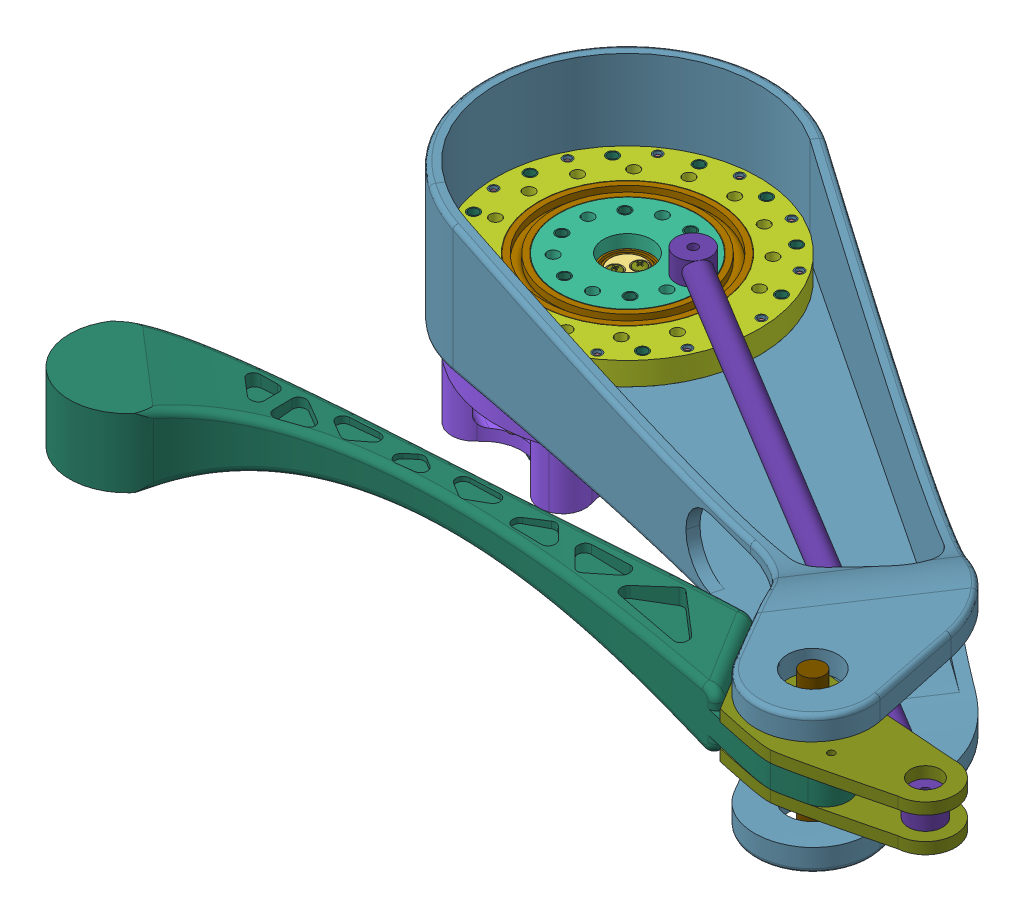
SolidWorks assembly Leg, configuration Default. Lengths in mm. (continued)
Components (placement in the parent): (continued)
- Cycloidal-1: Cycloidal [Default] at (-40.1687 29.4235 207.1731) x (-0.342839 0 -0.939394) z (0.939394 0 -0.342839) size (162.63 70.39 162.63) (continued)
  - M3x4x4.2_brass_insert-22: M3x4x4.2_brass_insert [Default] at (44.6897 69.6573 86.0997) x (0.984609 0 -0.174769) z (0.174769 0 0.984609) size (4 4 4)
  - M3x4x4.2_brass_insert-23: M3x4x4.2_brass_insert [Default] at (49.8443 69.6573 92.2177) x (0.984609 0 -0.174769) z (0.174769 0 0.984609) size (4 4 4)
  - pan cross head_am-4: pan cross head_am [B18.6.7M - M3 x 0.5 x 10 Type I Cross Recessed PHMS --10N] at (57.2541 77.5573 101.0123) x (0 -1 0) z (0 0 1) size (12.37 5.6 5.6)
  - pan cross head_am-5: pan cross head_am [B18.6.7M - M3 x 0.5 x 10 Type I Cross Recessed PHMS --10N] at (37.2799 77.5573 77.3051) x (0 -1 0) z (0 0 1) size (12.37 5.6 5.6)
  - pan cross head_am-6: pan cross head_am [B18.6.7M - M3 x 0.5 x 10 Type I Cross Recessed PHMS --10N] at (59.1206 77.5573 79.1715) x (0 -1 0) z (0 0 1) size (12.37 5.6 5.6)
  - pan cross head_am-7: pan cross head_am [B18.6.7M - M3 x 0.5 x 10 Type I Cross Recessed PHMS --10N] at (35.4134 77.5573 99.1458) x (0 -1 0) z (0 0 1) size (12.37 5.6 5.6)
  - radial ball bearing_68_iso-44: radial ball bearing_68_iso [ISO 15 RBB - 1715 - 26,SI,NC,26_68] at (46.1199 84.6573 90.1252) x (0 1 0) z (-0.714953 0 -0.699173) size (4 21 21)
  - radial ball bearing_68_iso-45: radial ball bearing_68_iso [ISO 15 RBB - 1715 - 26,SI,NC,26_68] at (47.267 89.6573 89.1587) x (0 1 0) z (0.999483 0 -0.032163) size (4 21 21)
  - radial ball bearing_68_iso-46: radial ball bearing_68_iso [ISO 15 RBB - 1715 - 26,SI,NC,26_68] at (48.4141 79.6573 88.1922) x (0 1 0) z (0 0 1) size (4 21 21)
  - socket button head screw_iso-37: socket button head screw_iso [ISO 7380 - M4 x 12 - 12N] at (79.0868 67.4573 57.3389) x (0 1 0) z (-0.709975 0 0.704227) size (14.2 7.6 7.6)
  - socket button head screw_iso-38: socket button head screw_iso [ISO 7380 - M4 x 12 - 12N] at (64.4877 67.4573 130.7332) x (0 1 0) z (-0.724148 0 0.689645) size (14.2 7.6 7.6)
  - foc-motor-controller.step-1: foc-motor-controller.step [Default] at (47.267 33.6573 89.1587) x (0.707107 0 0.707107) z (0 -1 0) size (57.23 50 8.13)
    - RTA0040B.step-1: RTA0040B.step [Default] at (12.5014 -1.6986 1.595) x (-0.707107 -0.707107 0) z (0 0 1) size (6 6 1)
      - FRAME.step-1: FRAME.step [Default] x (1 0 0) z (0 -1 0) size (6 0.2 6)
        - SOLID.step-1: SOLID.step [Default] at origin size (0.4 0.2 0.22)
        - SOLID-0.step-1: SOLID-0.step [Default] at origin size (0.4 0.2 0.22)
        - SOLID-1.step-1: SOLID-1.step [Default] at origin size (0.4 0.2 0.22)
        - SOLID-2.step-1: SOLID-2.step [Default] at origin size (0.4 0.2 0.22)
        - SOLID-3.step-1: SOLID-3.step [Default] at origin size (0.4 0.2 0.22)
        - SOLID-4.step-1: SOLID-4.step [Default] at origin size (0.4 0.2 0.22)
        - SOLID-5.step-1: SOLID-5.step [Default] at origin size (0.4 0.2 0.22)
        - SOLID-6.step-1: SOLID-6.step [Default] at origin size (0.4 0.2 0.22)
        - SOLID-7.step-1: SOLID-7.step [Default] at origin size (0.4 0.2 0.22)
        - SOLID-8.step-1: SOLID-8.step [Default] at origin size (0.4 0.2 0.22)
        - SOLID-9.step-1: SOLID-9.step [Default] at origin size (0.22 0.2 0.4)
        - SOLID-10.step-1: SOLID-10.step [Default] at origin size (0.22 0.2 0.4)
        - SOLID-11.step-1: SOLID-11.step [Default] at origin size (0.22 0.2 0.4)
        - SOLID-12.step-1: SOLID-12.step [Default] at origin size (0.22 0.2 0.4)
        - SOLID-13.step-1: SOLID-13.step [Default] at origin size (0.22 0.2 0.4)
        - SOLID-14.step-1: SOLID-14.step [Default] at origin size (0.22 0.2 0.4)
        - SOLID-15.step-1: SOLID-15.step [Default] at origin size (0.22 0.2 0.4)
        - SOLID-16.step-1: SOLID-16.step [Default] at origin size (0.22 0.2 0.4)
        - SOLID-17.step-1: SOLID-17.step [Default] at origin size (4.15 0.2 4.15)
        - SOLID-18.step-1: SOLID-18.step [Default] at origin size (0.28 0.1 0.28)
        - SOLID-19.step-1: SOLID-19.step [Default] at origin size (0.28 0.1 0.28)
        - SOLID-20.step-1: SOLID-20.step [Default] at origin size (0.28 0.1 0.28)
        - SOLID-21.step-1: SOLID-21.step [Default] at origin size (0.28 0.1 0.28)
        - SOLID-22.step-1: SOLID-22.step [Default] at origin size (0.4 0.2 0.22)
        - SOLID-23.step-1: SOLID-23.step [Default] at origin size (0.4 0.2 0.22)
        - SOLID-24.step-1: SOLID-24.step [Default] at origin size (0.4 0.2 0.22)
        - SOLID-25.step-1: SOLID-25.step [Default] at origin size (0.4 0.2 0.22)
        - SOLID-26.step-1: SOLID-26.step [Default] at origin size (0.4 0.2 0.22)
        - SOLID-27.step-1: SOLID-27.step [Default] at origin size (0.4 0.2 0.22)
        - SOLID-28.step-1: SOLID-28.step [Default] at origin size (0.4 0.2 0.22)
        - SOLID-29.step-1: SOLID-29.step [Default] at origin size (0.4 0.2 0.22)
        - SOLID-30.step-1: SOLID-30.step [Default] at origin size (0.4 0.2 0.22)
        - SOLID-31.step-1: SOLID-31.step [Default] at origin size (0.4 0.2 0.22)
        - SOLID-32.step-1: SOLID-32.step [Default] at origin size (0.22 0.2 0.4)
        - SOLID-33.step-1: SOLID-33.step [Default] at origin size (0.22 0.2 0.4)
        - SOLID-34.step-1: SOLID-34.step [Default] at origin size (0.22 0.2 0.4)
        - SOLID-35.step-1: SOLID-35.step [Default] at origin size (0.22 0.2 0.4)
        - SOLID-36.step-1: SOLID-36.step [Default] at origin size (0.22 0.2 0.4)
        - SOLID-37.step-1: SOLID-37.step [Default] at origin size (0.22 0.2 0.4)
        - SOLID-38.step-1: SOLID-38.step [Default] at origin size (0.22 0.2 0.4)
        - SOLID-39.step-1: SOLID-39.step [Default] at origin size (0.22 0.2 0.4)
        - SOLID-40.step-1: SOLID-40.step [Default] at origin size (0.22 0.2 0.4)
        - SOLID-41.step-1: SOLID-41.step [Default] at origin size (0.22 0.2 0.4)
        - SOLID-42.step-1: SOLID-42.step [Default] at origin size (0.22 0.2 0.4)
        - SOLID-43.step-1: SOLID-43.step [Default] at origin size (0.22 0.2 0.4)
      - BODY.step-1: BODY.step [Default] at (0 0 0.025) x (1 0 0) z (0 -1 0) size (6 0.97 6)
    - Resonator_SMD_Murata_CSTxExxV-3Pin_3.0x1.1mm.step-1: Resonator_SMD_Murata_CSTxExxV-3Pin_3.0x1.1mm.step [Default] at (1.8 -7 1.595) x (0 1 0) z (0 0 1) size (3.2 1.35 0.9)
    - C_0603_1608Metric.step-1: C_0603_1608Metric.step [Default] at (6.2 -16.8 1.595) x (0 -1 0) z (0 0 1) size (1.6 0.8 0.8)
    - R_0603_1608Metric.step-1: R_0603_1608Metric.step [Default] at (11.8 -7.375 1.595) x (0 1 0) z (0 0 1) size (1.6 0.8 0.45)
    - R_0603_1608Metric.step-2: R_0603_1608Metric.step [Default] at (13.8 -16.8 1.595) x (0 1 0) z (0 0 1) size (1.6 0.8 0.45)
    - R_0603_1608Metric.step-3: R_0603_1608Metric.step [Default] at (18.1 -5.36 1.595) size (1.6 0.8 0.45)
    - C_0603_1608Metric.step-2: C_0603_1608Metric.step [Default] at (2.6 -0.5 1.595) x (0 -1 0) z (0 0 1) size (1.6 0.8 0.8)
    - R_0603_1608Metric.step-4: R_0603_1608Metric.step [Default] at (14.6 -11.3 1.595) x (0 1 0) z (0 0 1) size (1.6 0.8 0.45)
    - L_APV_ANR4020.step-1: L_APV_ANR4020.step [Default] at (22.3 -13.7 1.595) x (0 -1 0) z (0 0 1) size (4.02 4 2)
    - C_0603_1608Metric.step-3: C_0603_1608Metric.step [Default] at (0.3 -12.6 1.595) x (-1 0 0) z (0 0 1) size (1.6 0.8 0.8)
    - C_1206_3216Metric.step-1: C_1206_3216Metric.step [Default] at (15.7 11 1.595) x (0 1 0) z (0 0 1) size (3.2 1.6 1.6)
    - C_0603_1608Metric.step-4: C_0603_1608Metric.step [Default] at (0.3 -9.6 1.595) size (1.6 0.8 0.8)
    - R_0603_1608Metric.step-5: R_0603_1608Metric.step [Default] at (12.3 -16.8 1.595) x (0 1 0) z (0 0 1) size (1.6 0.8 0.45)
    - C_0603_1608Metric.step-5: C_0603_1608Metric.step [Default] at (-0.3 -16.6 1.595) x (0 1 0) z (0 0 1) size (1.6 0.8 0.8)
    - R_0603_1608Metric.step-6: R_0603_1608Metric.step [Default] at (10.9 4.1 1.595) size (1.6 0.8 0.45)
    - C_1206_3216Metric.step-2: C_1206_3216Metric.step [Default] at (6.3 11 1.595) x (0 1 0) z (0 0 1) size (3.2 1.6 1.6)
    - XT30PW_2_2_-M.G.B.step-1: XT30PW_2_2_-M.G.B.step [Default] at (-20.5 9.5 1.595) x (0 -1 0) z (-1 0 0) size (15.5 7.1 12.53)
    - R_0603_1608Metric.step-7: R_0603_1608Metric.step [Default] at (0.3 -11.1 1.595) size (1.6 0.8 0.45)
    - C_0603_1608Metric.step-6: C_0603_1608Metric.step [Default] at (19 -0.4 1.595) x (-0.707107 -0.707107 0) z (0 0 1) size (1.6 0.8 0.8)
    - C_1206_3216Metric.step-3: C_1206_3216Metric.step [Default] at (13.3 11 1.595) x (0 1 0) z (0 0 1) size (3.2 1.6 1.6)
    - R_0603_1608Metric.step-8: R_0603_1608Metric.step [Default] at (10.2 -7.375 1.595) x (0 -1 0) z (0 0 1) size (1.6 0.8 0.45)
    - JST_GH_SM08B-GHS-TB_1x08-1MP_P1.25mm_Horizontal.step-1: JST_GH_SM08B-GHS-TB_1x08-1MP_P1.25mm_Horizontal.step [Default] at (10 -22 1.595) size (13.25 4.95 4.25)
    - C_1206_3216Metric.step-4: C_1206_3216Metric.step [Default] at (-12.3 11 1.595) x (0 1 0) z (0 0 1) size (3.2 1.6 1.6)
    - JST_GH_SM06B-GHS-TB_1x06-1MP_P1.25mm_Horizontal.step-1: JST_GH_SM06B-GHS-TB_1x06-1MP_P1.25mm_Horizontal.step [Default] at (-4.3 -22 1.595) size (10.75 4.95 4.25)
    - C_0603_1608Metric.step-7: C_0603_1608Metric.step [Default] at (7.3 -4.5 1.595) x (-1 0 0) z (0 0 1) size (1.6 0.8 0.8)
    - R_0603_1608Metric.step-9: R_0603_1608Metric.step [Default] at (18.1 -3.86 1.595) x (-1 0 0) z (0 0 1) size (1.6 0.8 0.45)
    - C_1206_3216Metric.step-5: C_1206_3216Metric.step [Default] at (22.6794 -1.2206 1.595) x (0.707107 -0.707107 0) z (0 0 1) size (3.2 1.6 1.6)
    - R_Array_Convex_4x0402.step-1: R_Array_Convex_4x0402.step [Default] at (6.8 -2.5 1.595) size (1 2 0.35)
    - R_0603_1608Metric.step-10: R_0603_1608Metric.step [Default] at (7.7 -16.8 1.595) x (0 -1 0) z (0 0 1) size (1.6 0.8 0.45)
    - C_1206_3216Metric.step-6: C_1206_3216Metric.step [Default] at (8.7 11 1.595) x (0 1 0) z (0 0 1) size (3.2 1.6 1.6)
    - C_0603_1608Metric.step-8: C_0603_1608Metric.step [Default] at (16.1 -11.3 1.595) x (0 1 0) z (0 0 1) size (1.6 0.8 0.8)
    - SOT-23-5.step-1: SOT-23-5.step [Default] at (-3.1 -16.6 1.595) x (-1 0 0) z (0 0 1) size (2.8 2.9 1.55)
    - C_0603_1608Metric.step-9: C_0603_1608Metric.step [Default] at (17.8 -13.6 1.595) size (1.6 0.8 0.8)
    - R_0603_1608Metric.step-11: R_0603_1608Metric.step [Default] at (-11.5 -20.3875 1.595) x (0 -1 0) z (0 0 1) size (1.6 0.8 0.45)
    - C_0603_1608Metric.step-10: C_0603_1608Metric.step [Default] at (-12.4 2.3 1.595) x (0 1 0) z (0 0 1) size (1.6 0.8 0.8)
    - C_1206_3216Metric.step-7: C_1206_3216Metric.step [Default] at (18 11 1.595) x (0 1 0) z (0 0 1) size (3.2 1.6 1.6)
    - R_0603_1608Metric.step-12: R_0603_1608Metric.step [Default] at (-10.8105 -14.9971 1.595) x (-1 0 0) z (0 0 1) size (1.6 0.8 0.45)
    - C_0603_1608Metric.step-11: C_0603_1608Metric.step [Default] at (-13.8 -9.4 1.595) x (-1 0 0) z (0 0 1) size (1.6 0.8 0.8)
    - R_0603_1608Metric.step-13: R_0603_1608Metric.step [Default] at (-23.15 -14.5 1.595) x (-1 0 0) z (0 0 1) size (1.6 0.8 0.45)
    - C_0603_1608Metric.step-12: C_0603_1608Metric.step [Default] at (1.1 -0.2 1.595) x (0 1 0) z (0 0 1) size (1.6 0.8 0.8)
    - D_0805_2012Metric.step-1: D_0805_2012Metric.step [Default] at (22.9 -9.6 1.595) x (0 1 0) z (0 0 1) size (2 1.27 0.8)
    - C_0603_1608Metric.step-13: C_0603_1608Metric.step [Default] at (-7.8 3.775 1.595) x (0 -1 0) z (0 0 1) size (1.6 0.8 0.8)
    - R_0603_1608Metric.step-14: R_0603_1608Metric.step [Default] at (-6.4 -12.825 1.595) x (0 1 0) z (0 0 1) size (1.6 0.8 0.45)
    - L_0603_1608Metric.step-1: L_0603_1608Metric.step [Default] at (-10.1 3 1.595) size (1.6 0.8 0.8)
    - C_0603_1608Metric.step-14: C_0603_1608Metric.step [Default] at (17.9 0.7 1.595) x (-0.707107 -0.707107 0) z (0 0 1) size (1.6 0.8 0.8)
    - HVSSOP-10.step-1: HVSSOP-10.step [Default] at (18.6 -9.6 1.595) x (0 -1 0) z (-1 0 0) size (4.9 1.1 3)
    - C_0603_1608Metric.step-15: C_0603_1608Metric.step [Default] at (7.9 4.1 1.595) x (-1 0 0) z (0 0 1) size (1.6 0.8 0.8)
    - C_0603_1608Metric.step-16: C_0603_1608Metric.step [Default] at (21.1 -9.6 1.595) x (0 -1 0) z (0 0 1) size (1.6 0.8 0.8)
    - R_0603_1608Metric.step-15: R_0603_1608Metric.step [Default] at (-10.8105 -11.9971 1.595) x (-1 0 0) z (0 0 1) size (1.6 0.8 0.45)
    - R_0603_1608Metric.step-16: R_0603_1608Metric.step [Default] at (-18.2 -17.4 1.595) size (1.6 0.8 0.45)
    - C_1206_3216Metric.step-8: C_1206_3216Metric.step [Default] at (-3 11 1.595) x (0 1 0) z (0 0 1) size (3.2 1.6 1.6)
    - R_0603_1608Metric.step-17: R_0603_1608Metric.step [Default] at (-16.9 -20.4 1.595) x (0 -1 0) z (0 0 1) size (1.6 0.8 0.45)
    - R_0603_1608Metric.step-18: R_0603_1608Metric.step [Default] at (-13.3 -20.3875 1.595) x (0 -1 0) z (0 0 1) size (1.6 0.8 0.45)
    - R_0603_1608Metric.step-19: R_0603_1608Metric.step [Default] at (-15.1 -20.3875 1.595) x (0 -1 0) z (0 0 1) size (1.6 0.8 0.45)
    - C_0603_1608Metric.step-17: C_0603_1608Metric.step [Default] at (15.5 -14.4 1.595) x (0 -1 0) z (0 0 1) size (1.6 0.8 0.8)
    - LED_0603_1608Metric.step-1: LED_0603_1608Metric.step [Default] at (-11.5 -23.3875 1.595) x (0 1 0) z (0 0 1) size (1.6 0.8 1.1)
    - C_0805_2012Metric.step-1: C_0805_2012Metric.step [Default] at (19.95 -17 1.595) size (2 1.25 1.25)
    - D_SMB.step-1: D_SMB.step [Default] at (-16.5 11.208 1.595) x (0 -1 0) z (0 0 1) size (5.3 3.55 2.15)
    - C_1206_3216Metric.step-9: C_1206_3216Metric.step [Default] at (-5.3 11 1.595) x (0 1 0) z (0 0 1) size (3.2 1.6 1.6)
    - XT30PW_2_2_-M.G.B.step-2: XT30PW_2_2_-M.G.B.step [Default] at (-20.5 -6.5 1.595) x (0 -1 0) z (-1 0 0) size (15.5 7.1 12.53)
    - C_1206_3216Metric.step-10: C_1206_3216Metric.step [Default] at (1.7 11 1.595) x (0 1 0) z (0 0 1) size (3.2 1.6 1.6)
    - C_1206_3216Metric.step-11: C_1206_3216Metric.step [Default] at (11 11 1.595) x (0 1 0) z (0 0 1) size (3.2 1.6 1.6)
    - C_0603_1608Metric.step-18: C_0603_1608Metric.step [Default] at (-6.3 3.775 1.595) x (0 -1 0) z (0 0 1) size (1.6 0.8 0.8)
    - C_0603_1608Metric.step-19: C_0603_1608Metric.step [Default] at (16.8686 1.7314 1.595) x (0.707107 0.707107 0) z (0 0 1) size (1.6 0.8 0.8)
    - C_0603_1608Metric.step-20: C_0603_1608Metric.step [Default] at (-15.0105 -11.1 1.595) size (1.6 0.8 0.8)
    - C_1206_3216Metric.step-12: C_1206_3216Metric.step [Default] at (-7.7 11 1.595) x (0 1 0) z (0 0 1) size (3.2 1.6 1.6)
    - C_0603_1608Metric.step-21: C_0603_1608Metric.step [Default] at (-18.2 -15.8 1.595) size (1.6 0.8 0.8)
    - C_0603_1608Metric.step-22: C_0603_1608Metric.step [Default] at (-2.1 -11.3 1.595) x (0 -1 0) z (0 0 1) size (1.6 0.8 0.8)
    - C_0603_1608Metric.step-23: C_0603_1608Metric.step [Default] at (-10.8105 -13.4971 1.595) size (1.6 0.8 0.8)
    - C_1206_3216Metric.step-13: C_1206_3216Metric.step [Default] at (4 11 1.595) x (0 1 0) z (0 0 1) size (3.2 1.6 1.6)
    - R_0603_1608Metric.step-20: R_0603_1608Metric.step [Default] at (16 -17.8 1.595) x (0 1 0) z (0 0 1) size (1.6 0.8 0.45)
    - Texas_S-PVSON-N8.step-1: Texas_S-PVSON-N8.step [Default] at (-14.4105 -13.7 1.595) x (-1 0 0) z (0 0 1) size (3 2.98 0.92)
    - C_1206_3216Metric.step-14: C_1206_3216Metric.step [Default] at (21 -2.9 1.595) x (0.707107 -0.707107 0) z (0 0 1) size (3.2 1.6 1.6)
    - C_0603_1608Metric.step-24: C_0603_1608Metric.step [Default] at (-5.9 -16.6 1.595) x (0 1 0) z (0 0 1) size (1.6 0.8 0.8)
    - C_0603_1608Metric.step-25: C_0603_1608Metric.step [Default] at (-3.1 -14.1 1.595) size (1.6 0.8 0.8)
    - R_0603_1608Metric.step-21: R_0603_1608Metric.step [Default] at (7.2 -7.375 1.595) x (0 -1 0) z (0 0 1) size (1.6 0.8 0.45)
    - C_1206_3216Metric.step-15: C_1206_3216Metric.step [Default] at (-0.7 11 1.595) x (0 1 0) z (0 0 1) size (3.2 1.6 1.6)
    - LQFP-64_10x10mm_P0.5mm.step-1: LQFP-64_10x10mm_P0.5mm.step [Default] at (-7 -4.5 1.595) x (-1 0 0) z (0 0 1) size (12 12 1.5)
    - C_0805_2012Metric.step-2: C_0805_2012Metric.step [Default] at (23.35 -17 1.595) x (-1 0 0) z (0 0 1) size (2 1.25 1.25)
    - C_0603_1608Metric.step-26: C_0603_1608Metric.step [Default] at (10.8 -16.8 1.595) x (0 -1 0) z (0 0 1) size (1.6 0.8 0.8)
    - R_0603_1608Metric.step-22: R_0603_1608Metric.step [Default] at (17.5 -17.8 1.595) x (0 -1 0) z (0 0 1) size (1.6 0.8 0.45)
    - C_1206_3216Metric.step-16: C_1206_3216Metric.step [Default] at (20.3 11 1.595) x (0 1 0) z (0 0 1) size (3.2 1.6 1.6)
    - R_0603_1608Metric.step-23: R_0603_1608Metric.step [Default] at (9.2 -16.8 1.595) x (0 -1 0) z (0 0 1) size (1.6 0.8 0.45)
    - C_1206_3216Metric.step-17: C_1206_3216Metric.step [Default] at (-10 11 1.595) x (0 1 0) z (0 0 1) size (3.2 1.6 1.6)
    - R_0603_1608Metric.step-24: R_0603_1608Metric.step [Default] at (17.8 -15.2 1.595) size (1.6 0.8 0.45)
    - C_1206_3216Metric.step-18: C_1206_3216Metric.step [Default] at (19.9 2.6 1.595) x (-0.707107 0.707107 0) z (0 0 1) size (3.2 1.6 1.6)
    - C_0603_1608Metric.step-27: C_0603_1608Metric.step [Default] at (13.4 -7.375 1.595) x (0 -1 0) z (0 0 1) size (1.6 0.8 0.8)
    - R_0603_1608Metric.step-25: R_0603_1608Metric.step [Default] at (8.7 -7.375 1.595) x (0 -1 0) z (0 0 1) size (1.6 0.8 0.45)
    - PQFN-8-EP_6x5mm_P1.27mm_Generic.step-1: PQFN-8-EP_6x5mm_P1.27mm_Generic.step [Default] at (4.9 14.4 -0.085) x (0 1 0) z (0 0 -1) size (6.15 5.15 1.09)
    - C_0805_2012Metric.step-3: C_0805_2012Metric.step [Default] at (-3 8.9 -0.085) x (0 1 0) z (0 0 -1) size (2 1.25 1.25)
    - C_0603_1608Metric.step-28: C_0603_1608Metric.step [Default] at (1.5 -4.3 -0.085) x (0 1 0) z (0 0 -1) size (1.6 0.8 0.8)
    - R_2512_6332Metric.step-1: R_2512_6332Metric.step [Default] at (2.1 8.6 -0.085) x (-1 0 0) z (0 0 -1) size (6.3 3.2 0.6)
    - C_0805_2012Metric.step-4: C_0805_2012Metric.step [Default] at (18.8 8.9 -0.085) x (0 1 0) z (0 0 -1) size (2 1.25 1.25)
    - C_0805_2012Metric.step-5: C_0805_2012Metric.step [Default] at (-5.2 8.901 -0.085) x (0 1 0) z (0 0 -1) size (2 1.25 1.25)
    - PQFN-8-EP_6x5mm_P1.27mm_Generic.step-2: PQFN-8-EP_6x5mm_P1.27mm_Generic.step [Default] at (16.9 14.6 -0.085) x (0 -1 0) z (0 0 -1) size (6.15 5.15 1.09)
    - PQFN-8-EP_6x5mm_P1.27mm_Generic.step-3: PQFN-8-EP_6x5mm_P1.27mm_Generic.step [Default] at (-1.1 14.6 -0.085) x (0 -1 0) z (0 0 -1) size (6.15 5.15 1.09)
    - R_0603_1608Metric.step-26: R_0603_1608Metric.step [Default] at (8.2 8.8 -0.085) x (0 1 0) z (0 0 -1) size (1.6 0.8 0.45)
    - R_2512_6332Metric.step-2: R_2512_6332Metric.step [Default] at (-10.3 8.601 -0.085) x (1 0 0) z (0 0 -1) size (6.3 3.2 0.6)
    - TSSOP-16_4.4x5mm_P0.65mm.step-1: TSSOP-16_4.4x5mm_P0.65mm.step [Default] at (0 0 -0.085) x (-1 0 0) z (0 0 -1) size (6.4 5 1.1)
    - C_0603_1608Metric.step-29: C_0603_1608Metric.step [Default] at (0 -4.25 -0.085) x (0 1 0) z (0 0 -1) size (1.6 0.8 0.8)
    - PQFN-8-EP_6x5mm_P1.27mm_Generic.step-4: PQFN-8-EP_6x5mm_P1.27mm_Generic.step [Default] at (10.9 14.4 -0.085) x (0 1 0) z (0 0 -1) size (6.15 5.15 1.09)
    - R_2512_6332Metric.step-3: R_2512_6332Metric.step [Default] at (13.7 8.6 -0.085) x (1 0 0) z (0 0 -1) size (6.3 3.2 0.6)
    - PQFN-8-EP_6x5mm_P1.27mm_Generic.step-5: PQFN-8-EP_6x5mm_P1.27mm_Generic.step [Default] at (-13.1 14.401 -0.085) x (0 1 0) z (0 0 -1) size (6.15 5.15 1.09)
    - C_0603_1608Metric.step-30: C_0603_1608Metric.step [Default] at (-1.5 -4.3 -0.085) x (0 -1 0) z (0 0 -1) size (1.6 0.8 0.8)
    - PQFN-8-EP_6x5mm_P1.27mm_Generic.step-6: PQFN-8-EP_6x5mm_P1.27mm_Generic.step [Default] at (-7.1 14.601 -0.085) x (0 -1 0) z (0 0 -1) size (6.15 5.15 1.09)
    - foc-motor-controller_PCB.step-1: foc-motor-controller_PCB.step [Default] at origin size (50 50 1.51)
  - hex nut style 1 gradeab_iso-1: hex nut style 1 gradeab_iso [ISO - 4032 - M3 - W - N] at (47.267 33.6573 58.7531) x (1 0 0) z (0 -1 0) size (5.5 6.35 2.4)
- Leg_Upper-1: Leg_Upper [Default] at (27.3814 131.6808 132.2037) x (0.837613 0 0.546264) z (-0.546264 0 0.837613) size (365.5 85.59 139.24)
- Leg_Lower-1: Leg_Lower [Default] at (-66.6656 -50.32 4.2262) x (0.997281 0 -0.073696) z (0.073696 0 0.997281) size (364 58.72 76.23)
  - Leg_Lower-1: Leg_Lower [Default] at (305.3917 182.0008 303.1692) size (327.4 58.72 76.23)
  - Leg_Lower_2-1: Leg_Lower_2 [Default] at (305.3917 207.0008 303.1692) size (106.04 5 47.53)
  - Leg_Lower_2-2: Leg_Lower_2 [Default] at (305.3917 192.0008 303.1692) size (106.04 5 47.53)
- Link_Rod-1: Link_Rod [Default] at (49.376 126.6808 125.4777) x (0.85579 0 0.517324) z (-0.517324 0 0.85579) size (315 10 15)
- m10-1: m10 [Default] at (260.2379 131.6808 284.0649) x (1 0 0.000242) z (-0.000242 0 1) size (10 60 10)
Mates (geometry in assembly coordinates):
- Concentric1: concentric anti-aligned: cylinder of Cycloidal-1/Cover-1 through (27.3814 126.6808 132.2037) axis (0 -1 0) radius 57.5; cylinder of Leg_Upper-1 through (27.3814 101.6808 132.2037) axis (0 1 0) radius 57.5
- Concentric2: concentric aligned: cylinder of Leg_Upper-1 through (260.2379 101.6808 284.0649) axis (0 1 0) radius 11; cylinder of Leg_Lower-1/Leg_Lower_2-1 through (260.2379 136.6808 284.0649) axis (0 1 0) radius 5
- Coincident2: coincident anti-aligned: plane of Cycloidal-1/Output_Shaft-1 through (27.3814 126.6808 132.2037) normal (0 1 0); plane of Link_Rod-1 through (49.376 126.6808 125.4777) normal (0 -1 0)
- Concentric3: concentric anti-aligned: cylinder of Leg_Lower-1/Leg_Lower_2-1 through (306.1128 136.6808 280.6749) axis (0 1 0) radius 6.5; cylinder of Link_Rod-1 through (306.1128 136.6808 280.6749) axis (0 -1 0) radius 2
- Coincident4: coincident anti-aligned: plane of Leg_Lower-1/Leg_Lower_2-1 through (260.2379 136.6808 284.0649) normal (0 -1 0); plane of Link_Rod-1 through (306.1128 136.6808 280.6749) normal (0 1 0)
- Concentric4: concentric aligned: cylinder of Cycloidal-1/M4x6x5.5_brass_insert-11 through (49.376 126.6808 125.4777) axis (0 -1 0) radius 2; cylinder of Link_Rod-1 through (49.376 136.6808 125.4777) axis (0 -1 0) radius 2
- Concentric5: concentric aligned: cylinder of Leg_Lower-1/Leg_Lower-1 through (260.2379 116.6808 284.0649) axis (0 1 0) radius 5; cylinder of m10-1 through (260.2379 101.6808 284.0649) axis (0 1 0) radius 5
- Coincident5: coincident aligned: plane of Leg_Lower-1/Leg_Lower-1 through (260.2379 131.6808 284.0649) normal (0 1 0); plane of m10-1 through (260.2379 131.6808 284.0649) normal (0 1 0)
- Coincident6: coincident aligned: plane of Leg_Upper-1 through (27.3814 161.6808 132.2037) normal (0 1 0); plane of m10-1 through (260.2379 161.6808 284.0649) normal (0 1 0)
